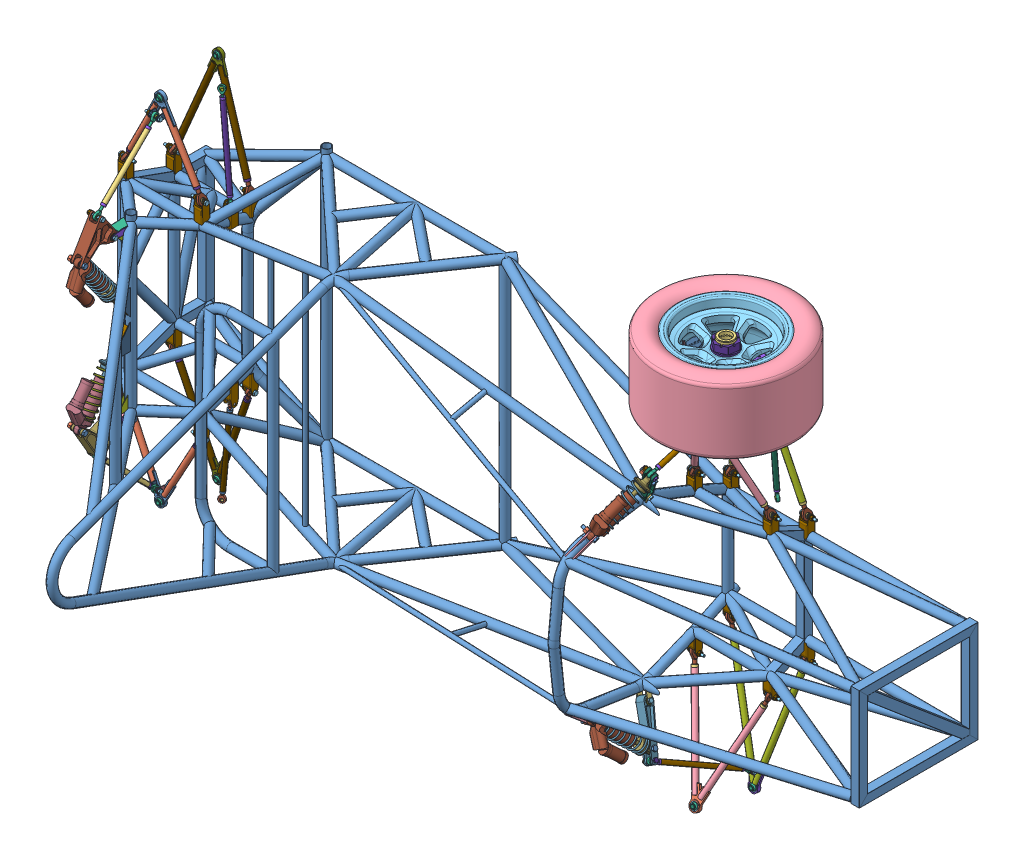
SolidWorks assembly AE-Rolling Chassis Assembly, configuration Default. Lengths in mm.
Overall size (2356.42 1252.94 1211.91).
496 component instances, 112 part files, 12 mates.
Components (placement in the parent):
- FR-A0100-FG_3-Space_Frame-1: FR-A0100-FG_3-Space_Frame [Default<As Machined>] at origin size (2341.42 791.46 1187.78)
- SP-A0200-AD-Front Axle Assembly-1: SP-A0200-AD-Front Axle Assembly [Default] at (231.003 -38.1001 -73.813) x (1 0 0) z (0 0 1) size (283.43 1142.4 502.75)
  - Upper A-Arm^SP-A0200-AD-Front Axle Assembly-1: Upper A-Arm^SP-A0200-AD-Front Axle Assembly [Default] at (0 340.1778 -103.3743) x (1 0 0) z (0 -0.807933 0.589274) size (223.78 263.64 179.68) (virtual)
    - SP-Upper Apex Front-1: SP-Upper Apex Front [Default] at (789.6198 444.1063 49.8797) x (0.938572 -0.289882 0.187221) z (0 0.542537 0.840032) size (51.11 64.07 9.53)
    - SP-10003-AD-Threaded Insert-1: SP-10003-AD-Threaded Insert [A-Arm] at (690.6588 218.0055 195.9078) x (-0.938572 0.289882 -0.187221) z (-0.345084 -0.78843 0.50921) size (15.88 15.88 15.88)
    - SP-10003-AD-Threaded Insert-2: SP-10003-AD-Threaded Insert [A-Arm] at (888.5808 218.0055 195.9078) x (0 0.542537 0.840032) z (0.345084 -0.78843 0.50921) size (15.88 15.88 15.88)
    - SP-Upper A-Arm Tube-1: SP-Upper A-Arm Tube [Default] at (732.4698 313.533 134.2109) x (0 -0.542537 -0.840032) z (0.938572 -0.289882 0.187221) size (15.88 272.31 15.88)
    - SP-Upper A-Arm Tube-2: SP-Upper A-Arm Tube [Default] at (846.7698 313.533 134.2109) x (0 0.542537 0.840032) z (-0.938572 -0.289882 0.187221) size (15.88 272.31 15.88)
    - FS-HIGH MISALIGN SPHERICAL BEARING, 0.375-0.906D (3072-6G)-1: FS-HIGH MISALIGN SPHERICAL BEARING, 0.375-0.906D (3072-6G) [Default] at (789.6198 444.1063 49.8797) x (-0.345084 -0.78843 0.50921) z (-0.938572 0.289882 -0.187221) size (26.46 21.71 26.13)
      - Race^FS-HIGH MISALIGN SPHERICAL BEARING, 0.375-0.906D (3072-6G)-1: Race^FS-HIGH MISALIGN SPHERICAL BEARING, 0.375-0.906D (3072-6G) [Default] at origin size (23.01 8.76 23.01) (virtual)
      - Ball^FS-HIGH MISALIGN SPHERICAL BEARING, 0.375-0.906D (3072-6G)-1: Ball^FS-HIGH MISALIGN SPHERICAL BEARING, 0.375-0.906D (3072-6G) [Default] x (0.359576 -0.008176 0.93308) z (-0.932238 -0.046516 0.358844) size (19.84 20.65 19.84) (virtual)
  - Lower A-Arm^SP-A0200-AD-Front Axle Assembly-1: Lower A-Arm^SP-A0200-AD-Front Axle Assembly [Default] at (0 -0.114 0.1797) x (1 0 0) z (0 0.000904 1) size (226.81 360.38 61.75) (virtual)
    - SP-Front Lower A-Arm Tube-2: SP-Front Lower A-Arm Tube [Default] at (844.893 441.1433 99.9128) x (0.296605 -0.948118 -0.114444) z (0 -0.119836 0.992794) size (339.15 15.88 15.88)
    - SP-Lower Apex Front-1: SP-Lower Apex Front [Default] at (798.1748 590.481 117.9388) x (0.955 -0.294468 -0.035544) z (0 -0.119836 0.992794) size (48.15 64.07 9.53)
    - SP-10003-AD-Threaded Insert-1: SP-10003-AD-Threaded Insert [A-Arm] at (899.2907 267.2577 78.9237) x (0.955 0.294468 0.035544) z (0.296605 -0.948118 -0.114444) size (15.88 15.88 15.88)
    - SP-10003-AD-Threaded Insert-2: SP-10003-AD-Threaded Insert [A-Arm] at (697.0589 267.2577 78.9237) x (0.955 -0.294468 -0.035544) z (-0.296605 -0.948118 -0.114444) size (15.88 15.88 15.88)
    - FS-HIGH MISALIGN SPHERICAL BEARING, 0.375-0.906D (3072-6G)-1: FS-HIGH MISALIGN SPHERICAL BEARING, 0.375-0.906D (3072-6G) [Default] at (798.1748 590.481 117.9388) x (0.296605 0.948118 0.114444) z (-0.955 0.294468 0.035544) size (26.46 21.71 26.13)
      - Race^FS-HIGH MISALIGN SPHERICAL BEARING, 0.375-0.906D (3072-6G)-1: Race^FS-HIGH MISALIGN SPHERICAL BEARING, 0.375-0.906D (3072-6G) [Default] at origin size (23.01 8.76 23.01) (virtual)
      - Ball^FS-HIGH MISALIGN SPHERICAL BEARING, 0.375-0.906D (3072-6G)-1: Ball^FS-HIGH MISALIGN SPHERICAL BEARING, 0.375-0.906D (3072-6G) [Default] x (0.359576 -0.008176 0.93308) z (-0.932238 -0.046516 0.358844) size (19.84 20.65 19.84) (virtual)
    - SP-Front Lower A-Arm Tube-3: SP-Front Lower A-Arm Tube [Default] at (751.4566 441.1433 99.9128) x (-0.296605 -0.948118 -0.114444) z (0 -0.119836 0.992794) size (339.15 15.88 15.88)
  - SP-C30066-AA-A-Arm Tab Box-2: SP-C30066-AA-A-Arm Tab Box [Default] at (903.9198 253.9613 173.2262) x (0 1 0) z (0 0 -1) size (60.32 25.4 25.4)
  - SP-C30066-AA-A-Arm Tab Box-3: SP-C30066-AA-A-Arm Tab Box [Default] at (675.3198 253.9613 173.2262) x (0 1 0) z (0 0 -1) size (60.32 25.4 25.4)
  - SP-C30066-AA-A-Arm Tab Box-4: SP-C30066-AA-A-Arm Tab Box [Default] at (912.4748 207.6041 73.8128) x (0 1 0) z (0 0 -1) size (60.32 25.4 25.4)
  - SP-C30066-AA-A-Arm Tab Box-5: SP-C30066-AA-A-Arm Tab Box [Default] at (683.8748 207.6066 73.5172) x (0 0.999857 0.016927) z (0 0.016927 -0.999857) size (60.32 25.4 25.4)
  - SP-30063-AB- Front Pushrod Tab-1: SP-30063-AB- Front Pushrod Tab [Default] at (810.0811 539.62 115.4288) x (1 0 0) z (0 0.104591 -0.994515) size (1.59 15.88 23.81)
  - SP-30063-AB- Front Pushrod Tab-2: SP-30063-AB- Front Pushrod Tab [Default] at (786.2686 539.62 115.4288) x (1 0 0) z (0 0.104591 -0.994515) size (1.59 15.88 23.81)
  - SP-A0105-AC-Ohlin TTX25 MKII, 200mm-2: SP-A0105-AC-Ohlin TTX25 MKII, 200mm [Default] at (696.4401 277.6233 502.0343) x (0.862886 -0.493364 -0.109636) z (-0.277169 -0.64335 0.713637) size (48.39 85.02 197.6)
    - Shock Body^SP-A0105-AC-Ohlin TTX25 MKII, 200mm-1: Shock Body^SP-A0105-AC-Ohlin TTX25 MKII, 200mm [Default] at origin size (40.76 80 131.7) (virtual)
    - Head^SP-A0105-AC-Ohlin TTX25 MKII, 200mm-1: Head^SP-A0105-AC-Ohlin TTX25 MKII, 200mm [Default] at (0 0 -174.6) size (46 46 119) (virtual)
    - Ball^SP-A0105-AC-Ohlin TTX25 MKII, 200mm-1: Ball^SP-A0105-AC-Ohlin TTX25 MKII, 200mm [Default] at (0 0 -174.6) x (-0.011681 0.107343 0.994153) z (0.993776 0.111394 -0.000351) size (15 15 8) (virtual)
    - Ball^SP-A0105-AC-Ohlin TTX25 MKII, 200mm-2: Ball^SP-A0105-AC-Ohlin TTX25 MKII, 200mm [Default] x (0.079523 -0.862756 -0.499328) z (0.965926 -0.057074 0.252448) size (15 15 8) (virtual)
    - SP-#####-AB-Spring-1: SP-#####-AB-Spring [Default] at (0 0 -151.1) size (48.39 49.05 127.97)
  - Front Rocker Assembly-1: Front Rocker Assembly [Default] at (694.2782 309.5507 341.3462) x (0.862886 -0.493364 -0.109636) z (-0.088476 -0.361041 0.928343) size (45.3 150.81 28.57)
    - SP-Front Rocker-1: SP-Front Rocker [Default] at origin size (25.4 150.81 28.57)
    - FS-BALL BEARING, 0.25ID-0.75OD (60355K702)-1: FS-BALL BEARING, 0.25ID-0.75OD (60355K702) [Default] at (9.1281 0 0) x (0 0 1) z (-1 0 0) size (19.05 19.05 7.14)
    - FS-BALL BEARING, 0.25ID-0.75OD (60355K702)-2: FS-BALL BEARING, 0.25ID-0.75OD (60355K702) [Default] at (-9.1281 0 0) x (0 0 1) z (-1 0 0) size (19.05 19.05 7.14)
    - FS-CADMIUM PLATED C3 HX, 0.25x28-1.41-0.469 (AN4-13A)-1: FS-CADMIUM PLATED C3 HX, 0.25x28-1.41-0.469 (AN4-13A) [Default] at (-3.0226 127 0) x (-1 0 0) z (0 1 0) size (40.18 12.9 11.18)
    - FS-NYLOC G8 HX, 0.25x28-0.3125 (90630A145)-1: FS-NYLOC G8 HX, 0.25x28-0.3125 (90630A145) [Default] at (-12.7 127 0) x (0 1 0) z (0 0 1) size (11.11 7.94 12.83)
    - FS-ZINC YELLOW CHROMATE C10.9 HX, M8x1.25-40-22 (95327A569)-1: FS-ZINC YELLOW CHROMATE C10.9 HX, M8x1.25-40-22 (95327A569) [Default] at (-4.65 101.6 0) x (-1 0 0) z (0 0 1) size (45.3 15.01 13)
    - FS-NYLOC FLHX C8, M8x1.25-11.1 (92461A400)-1: FS-NYLOC FLHX C8, M8x1.25-11.1 (92461A400) [Default] at (-23.8 101.6 0) x (0 1 0) z (-1 0 0) size (17.9 17.9 11.1)
  - SP-A0200-Front Rocker Tab Box-1: SP-A0200-Front Rocker Tab Box [Front] at (706.6066 302.5017 339.7797) x (0.862886 -0.493364 -0.109636) z (-0.497595 -0.791354 -0.355188) size (3.17 19.05 44.54)
  - SP-A0200-Front Rocker Tab Box-2: SP-A0200-Front Rocker Tab Box [Front] at (681.9497 316.5996 342.9126) x (0.862886 -0.493364 -0.109636) z (-0.497595 -0.791354 -0.355188) size (3.17 19.05 44.54)
  - SP-A0200-Shock Tab-1: SP-A0200-Shock Tab [Default] at (703.1358 273.795 501.1836) x (0.862886 -0.493364 -0.109636) z (-0.277169 -0.64335 0.713637) size (3.17 23.81 77.22)
  - SP-A0200-Shock Tab-2: SP-A0200-Shock Tab [Default] at (689.4375 281.6271 502.9241) x (0.862886 -0.493364 -0.109636) z (-0.277169 -0.64335 0.713637) size (3.17 23.81 77.22)
  - FS-NYLOC G8 HX, 0.25x28-0.3125 (90630A145)-3: FS-NYLOC G8 HX, 0.25x28-0.3125 (90630A145) [Default] at (688.0198 271.4238 173.2262) x (0 0 -1) z (0 -1 0) size (11.11 7.94 12.83)
  - FS-NYLOC G8 HX, 0.25x28-0.3125 (90630A145)-4: FS-NYLOC G8 HX, 0.25x28-0.3125 (90630A145) [Default] at (696.5748 225.0666 73.8128) x (0 0 1) z (0 1 0) size (11.11 7.94 12.83)
  - FS-CADMIUM PLATED C3 HEX, 0.25x28-1.65-0.469 (AN4-13A)-1: FS-CADMIUM PLATED C3 HEX, 0.25x28-1.65-0.469 (AN4-13A) [Default] at (909.9904 271.4238 173.2262) size (46.28 12.9 11.18)
  - FS-CADMIUM PLATED C3 HEX, 0.25x28-1.65-0.469 (AN4-13A)-2: FS-CADMIUM PLATED C3 HEX, 0.25x28-1.65-0.469 (AN4-13A) [Default] at (681.3904 271.4238 173.2262) size (46.28 12.9 11.18)
  - FS-CADMIUM PLATED C3 HEX, 0.25x28-1.65-0.469 (AN4-13A)-3: FS-CADMIUM PLATED C3 HEX, 0.25x28-1.65-0.469 (AN4-13A) [Default] at (689.9454 225.0666 73.8128) size (46.28 12.9 11.18)
  - FS-CADMIUM PLATED C3 HEX, 0.25x28-1.65-0.469 (AN4-13A)-4: FS-CADMIUM PLATED C3 HEX, 0.25x28-1.65-0.469 (AN4-13A) [Default] at (918.5454 225.0666 73.8128) size (46.28 12.9 11.18)
  - FS-CADMIUM PLATED C3 HEX, 0.25x28-1.65-0.469 (AN4-13A)-5: FS-CADMIUM PLATED C3 HEX, 0.25x28-1.65-0.469 (AN4-13A) [Default] at (792.898 537.9596 131.2167) x (-1 0 0) z (0 0.104591 -0.994515) size (46.28 12.9 11.18)
  - FS-CADMIUM PLATED C3 HEX, 0.25x28-1.65-0.469 (AN4-13A)-6: FS-CADMIUM PLATED C3 HEX, 0.25x28-1.65-0.469 (AN4-13A) [Default] at (691.7796 310.9792 341.6636) x (-0.862886 0.493364 0.109636) z (0.505399 0.842338 0.187186) size (46.28 12.9 11.18)
  - FS-ZINC YELLOW CHROMATE C10.9 HX, M8x1.25-40-22 (95327A569)-1: FS-ZINC YELLOW CHROMATE C10.9 HX, M8x1.25-40-22 (95327A569) [Default] at (689.5346 281.5716 502.9117) x (-0.862886 0.493364 0.109636) z (0.422618 0.5854 0.691883) size (45.3 15.01 13)
  - FS-NYLOC FLHX C8, M8x1.25-11.1 (92461A400)-1: FS-NYLOC FLHX C8, M8x1.25-11.1 (92461A400) [Default] at (678.4896 287.8867 504.3151) x (-0.277169 -0.64335 0.713637) z (-0.862886 0.493364 0.109636) size (17.9 17.9 11.1)
  - FS-NYLOC G8 HX, 0.25x28-0.3125 (90630A145)-1: FS-NYLOC G8 HX, 0.25x28-0.3125 (90630A145) [Default] at (916.6198 271.4238 173.2262) x (0 0 -1) z (0 -1 0) size (11.11 7.94 12.83)
  - FS-NYLOC G8 HX, 0.25x28-0.3125 (90630A145)-2: FS-NYLOC G8 HX, 0.25x28-0.3125 (90630A145) [Default] at (925.1748 225.0666 73.8128) x (0 0 1) z (0 1 0) size (11.11 7.94 12.83)
  - FS-NYLOC G8 HX, 0.25x28-0.3125 (90630A145)-5: FS-NYLOC G8 HX, 0.25x28-0.3125 (90630A145) [Default] at (786.2686 537.9596 131.2167) x (0 0.994515 0.104591) z (0 -0.104591 0.994515) size (11.11 7.94 12.83)
  - Push Rod^SP-A0200-AD-Front Axle Assembly-1: Push Rod^SP-A0200-AD-Front Axle Assembly [Default] at (-77.4197 117.9369 116.0221) x (0.981785 -0.1411 -0.127232) z (0.129346 0.005872 0.991582) size (77.15 168.18 273.97) (virtual)
    - FS-MALE ROD END UNF-3A, 0.25x28-0.25D (AM-4)-1: FS-MALE ROD END UNF-3A, 0.25x28-0.25D (AM-4) [Default] at (744.0599 398.8817 377.8613) x (-0.313321 -0.797417 -0.515709) z (0.188596 0.479987 -0.856764) size (19.32 14.06 49.44)
      - Body^FS-MALE ROD END UNF-3A, 0.25x28-0.25D (AM-4)-2: Body^FS-MALE ROD END UNF-3A, 0.25x28-0.25D (AM-4) [Default] at origin size (19.32 7.2 49.44) (virtual)
      - Ball^FS-MALE ROD END UNF-3A, 0.25x28-0.25D (AM-4)-2: Ball^FS-MALE ROD END UNF-3A, 0.25x28-0.25D (AM-4) [Default] x (0.09633 0.218783 0.971007) z (-0.984027 0.167661 0.059845) size (12.7 9.53 12.7) (virtual)
    - FS-MALE ROD END UNF-3A, 0.25x28-0.25D (AM-4)-2: FS-MALE ROD END UNF-3A, 0.25x28-0.25D (AM-4) [Default] at (798.4475 537.3007 130.7871) x (0.310336 0.78982 0.529034) z (-0.193469 -0.492388 0.848601) size (19.32 14.06 49.44)
      - Body^FS-MALE ROD END UNF-3A, 0.25x28-0.25D (AM-4)-2: Body^FS-MALE ROD END UNF-3A, 0.25x28-0.25D (AM-4) [Default] at origin size (19.32 7.2 49.44) (virtual)
      - Ball^FS-MALE ROD END UNF-3A, 0.25x28-0.25D (AM-4)-2: Ball^FS-MALE ROD END UNF-3A, 0.25x28-0.25D (AM-4) [Default] x (0.09633 0.218783 0.971007) z (-0.984027 0.167661 0.059845) size (12.7 9.53 12.7) (virtual)
    - SP-10003-AC-Threaded Insert-1: SP-10003-AC-Threaded Insert [AM-4 Rod End Thread] at (750.6466 415.6452 347.9388) x (0.313321 0.797417 0.515709) z (-0.188596 -0.479987 0.856764) size (12.7 12.7 15.88)
    - SP-10003-AC-Threaded Insert-2: SP-10003-AC-Threaded Insert [AM-4 Rod End Thread] at (791.691 520.1052 160.4226) x (-0.310336 -0.78982 -0.529034) z (0.193469 0.492388 -0.848601) size (12.7 12.7 15.88)
    - SP-A0200-Front Push Rod Tube-1: SP-A0200-Front Push Rod Tube [Default] at (771.2537 468.0912 254.3242) x (-0.313321 -0.797417 -0.515709) z (0.930732 -0.365703 0) size (12.7 237.68 12.7)
  - FS-ROD END RETAINING WASHER, 0.25-0.245 (NO PN)-1: FS-ROD END RETAINING WASHER, 0.25-0.245 (NO PN) [Default] at (923.7143 225.0666 73.8128) x (0 0 1) z (-1 0 0) size (12.7 12.7 6.22)
  - FS-ROD END RETAINING WASHER, 0.25-0.245 (NO PN)-2: FS-ROD END RETAINING WASHER, 0.25-0.245 (NO PN) [Default] at (901.2353 225.0666 73.8128) x (0 0 -1) z (1 0 0) size (12.7 12.7 6.22)
  - FS-ROD END RETAINING WASHER, 0.25-0.245 (NO PN)-3: FS-ROD END RETAINING WASHER, 0.25-0.245 (NO PN) [Default] at (915.1593 271.4238 173.2262) x (0 0 -1) z (-1 0 0) size (12.7 12.7 6.22)
  - FS-ROD END RETAINING WASHER, 0.25-0.245 (NO PN)-4: FS-ROD END RETAINING WASHER, 0.25-0.245 (NO PN) [Default] at (892.6803 271.4238 173.2262) x (0 0 1) z (1 0 0) size (12.7 12.7 6.22)
  - FS-ROD END RETAINING WASHER, 0.25-0.245 (NO PN)-5: FS-ROD END RETAINING WASHER, 0.25-0.245 (NO PN) [Default] at (695.1143 225.0666 73.8128) x (0 0 1) z (-1 0 0) size (12.7 12.7 6.22)
  - FS-ROD END RETAINING WASHER, 0.25-0.245 (NO PN)-6: FS-ROD END RETAINING WASHER, 0.25-0.245 (NO PN) [Default] at (672.6353 225.0666 73.8128) x (0 0 -1) z (1 0 0) size (12.7 12.7 6.22)
  - FS-ROD END RETAINING WASHER, 0.25-0.245 (NO PN)-7: FS-ROD END RETAINING WASHER, 0.25-0.245 (NO PN) [Default] at (686.5593 271.4238 173.2262) x (0 0 -1) z (-1 0 0) size (12.7 12.7 6.22)
  - FS-ROD END RETAINING WASHER, 0.25-0.245 (NO PN)-8: FS-ROD END RETAINING WASHER, 0.25-0.245 (NO PN) [Default] at (664.0803 271.4238 173.2262) x (0 0 1) z (1 0 0) size (12.7 12.7 6.22)
  - FS-ROD END RETAINING WASHER, 0.25-0.245 (NO PN)-9: FS-ROD END RETAINING WASHER, 0.25-0.245 (NO PN) [Default] at (810.2081 537.9596 131.2167) x (0 0.994515 0.104591) z (-1 0 0) size (12.7 12.7 6.22)
  - FS-ROD END RETAINING WASHER, 0.25-0.245 (NO PN)-10: FS-ROD END RETAINING WASHER, 0.25-0.245 (NO PN) [Default] at (787.7291 537.9596 131.2167) x (0 -0.994515 -0.104591) z (1 0 0) size (12.7 12.7 6.22)
  - FS-MALE ROD END UNJF-3A, 0.375x24-0.25D (HXAM-4T)-1: FS-MALE ROD END UNJF-3A, 0.375x24-0.25D (HXAM-4T) [Simplified] at (675.3198 271.4238 173.2262) x (0.013325 0.354377 -0.935008) z (0.345084 0.876009 0.336934) size (26.22 15.06 62.54)
    - Body^FS-MALE ROD END UNJF-3A, 0.375x24-0.25D (HXAM-4T)-1: Body^FS-MALE ROD END UNJF-3A, 0.375x24-0.25D (HXAM-4T) [no_threads] at origin size (26.22 9.62 62.54)
    - Ball^FS-MALE ROD END UNJF-3A, 0.375x24-0.25D (HXAM-4T)-1: Ball^FS-MALE ROD END UNJF-3A, 0.375x24-0.25D (HXAM-4T) [Default] at origin size (15.06 15.06 15.06)
  - FS-MALE ROD END UNJF-3A, 0.375x24-0.25D (HXAM-4T)-2: FS-MALE ROD END UNJF-3A, 0.375x24-0.25D (HXAM-4T) [Simplified] at (903.9198 271.4238 173.2262) x (0.045305 -0.343021 0.938235) z (-0.345084 0.876009 0.336934) size (26.22 15.06 62.54)
    - Body^FS-MALE ROD END UNJF-3A, 0.375x24-0.25D (HXAM-4T)-1: Body^FS-MALE ROD END UNJF-3A, 0.375x24-0.25D (HXAM-4T) [no_threads] at origin size (26.22 9.62 62.54)
    - Ball^FS-MALE ROD END UNJF-3A, 0.375x24-0.25D (HXAM-4T)-1: Ball^FS-MALE ROD END UNJF-3A, 0.375x24-0.25D (HXAM-4T) [Default] at origin size (15.06 15.06 15.06)
  - FS-MALE ROD END UNJF-3A, 0.375x24-0.25D (HXAM-4T)-3: FS-MALE ROD END UNJF-3A, 0.375x24-0.25D (HXAM-4T) [Simplified] at (683.8748 225.0666 73.8128) x (0.051295 0.102949 -0.993363) z (0.296605 0.948221 0.113586) size (26.22 15.06 62.54)
    - Body^FS-MALE ROD END UNJF-3A, 0.375x24-0.25D (HXAM-4T)-1: Body^FS-MALE ROD END UNJF-3A, 0.375x24-0.25D (HXAM-4T) [no_threads] at origin size (26.22 9.62 62.54)
    - Ball^FS-MALE ROD END UNJF-3A, 0.375x24-0.25D (HXAM-4T)-1: Ball^FS-MALE ROD END UNJF-3A, 0.375x24-0.25D (HXAM-4T) [Default] at origin size (15.06 15.06 15.06)
  - FS-MALE ROD END UNJF-3A, 0.375x24-0.25D (HXAM-4T)-4: FS-MALE ROD END UNJF-3A, 0.375x24-0.25D (HXAM-4T) [Simplified] at (912.4748 225.0666 73.8128) x (0.102858 0.149966 -0.983326) z (-0.296605 0.948221 0.113586) size (26.22 15.06 62.54)
    - Body^FS-MALE ROD END UNJF-3A, 0.375x24-0.25D (HXAM-4T)-1: Body^FS-MALE ROD END UNJF-3A, 0.375x24-0.25D (HXAM-4T) [no_threads] at origin size (26.22 9.62 62.54)
    - Ball^FS-MALE ROD END UNJF-3A, 0.375x24-0.25D (HXAM-4T)-1: Ball^FS-MALE ROD END UNJF-3A, 0.375x24-0.25D (HXAM-4T) [Default] at origin size (15.06 15.06 15.06)
  - FS-NYLOC G8 HX, 0.25x28-0.3125 (90630A145)-6: FS-NYLOC G8 HX, 0.25x28-0.3125 (90630A145) [Default] at (925.1748 -148.8666 73.8128) x (0 0 1) z (0 1 0) size (11.11 7.94 12.83)
  - FS-CADMIUM PLATED C3 HEX, 0.25x28-1.65-0.469 (AN4-13A)-7: FS-CADMIUM PLATED C3 HEX, 0.25x28-1.65-0.469 (AN4-13A) [Default] at (792.898 -461.7596 131.2167) x (-1 0 0) z (0 0.104591 0.994515) size (46.28 12.9 11.18)
  - FS-CADMIUM PLATED C3 HEX, 0.25x28-1.65-0.469 (AN4-13A)-8: FS-CADMIUM PLATED C3 HEX, 0.25x28-1.65-0.469 (AN4-13A) [Default] at (691.7796 -234.7792 341.6636) x (-0.862886 -0.493364 0.109636) z (-0.505399 0.842338 -0.187186) size (46.28 12.9 11.18)
  - FS-ROD END RETAINING WASHER, 0.25-0.245 (NO PN)-11: FS-ROD END RETAINING WASHER, 0.25-0.245 (NO PN) [Default] at (672.6353 -148.8666 73.8128) x (0 0 1) z (1 0 0) size (12.7 12.7 6.22)
  - FS-ROD END RETAINING WASHER, 0.25-0.245 (NO PN)-12: FS-ROD END RETAINING WASHER, 0.25-0.245 (NO PN) [Default] at (901.2353 -148.8666 73.8128) x (0 0 1) z (1 0 0) size (12.7 12.7 6.22)
  - FS-NYLOC G8 HX, 0.25x28-0.3125 (90630A145)-7: FS-NYLOC G8 HX, 0.25x28-0.3125 (90630A145) [Default] at (696.5748 -148.8666 73.8128) x (0 0 1) z (0 1 0) size (11.11 7.94 12.83)
  - FS-NYLOC FLHX C8, M8x1.25-11.1 (92461A400)-2: FS-NYLOC FLHX C8, M8x1.25-11.1 (92461A400) [Default] at (678.4896 -211.6867 504.3151) x (0.277169 -0.64335 -0.713637) z (-0.862886 -0.493364 0.109636) size (17.9 17.9 11.1)
  - FS-NYLOC G8 HX, 0.25x28-0.3125 (90630A145)-8: FS-NYLOC G8 HX, 0.25x28-0.3125 (90630A145) [Default] at (688.0198 -195.2238 173.2262) x (0 0 -1) z (0 -1 0) size (11.11 7.94 12.83)
  - FS-CADMIUM PLATED C3 HEX, 0.25x28-1.65-0.469 (AN4-13A)-9: FS-CADMIUM PLATED C3 HEX, 0.25x28-1.65-0.469 (AN4-13A) [Default] at (918.5454 -148.8666 73.8128) x (1 0 0) z (0 0 -1) size (46.28 12.9 11.18)
  - FS-CADMIUM PLATED C3 HEX, 0.25x28-1.65-0.469 (AN4-13A)-10: FS-CADMIUM PLATED C3 HEX, 0.25x28-1.65-0.469 (AN4-13A) [Default] at (909.9904 -195.2238 173.2262) x (1 0 0) z (0 0 -1) size (46.28 12.9 11.18)
  - FS-ROD END RETAINING WASHER, 0.25-0.245 (NO PN)-13: FS-ROD END RETAINING WASHER, 0.25-0.245 (NO PN) [Default] at (695.1143 -148.8666 73.8128) x (0 0 -1) z (-1 0 0) size (12.7 12.7 6.22)
  - FS-NYLOC G8 HX, 0.25x28-0.3125 (90630A145)-9: FS-NYLOC G8 HX, 0.25x28-0.3125 (90630A145) [Default] at (916.6198 -195.2238 173.2262) x (0 0 -1) z (0 -1 0) size (11.11 7.94 12.83)
  - FS-ROD END RETAINING WASHER, 0.25-0.245 (NO PN)-14: FS-ROD END RETAINING WASHER, 0.25-0.245 (NO PN) [Default] at (923.7143 -148.8666 73.8128) x (0 0 -1) z (-1 0 0) size (12.7 12.7 6.22)
  - FS-ROD END RETAINING WASHER, 0.25-0.245 (NO PN)-15: FS-ROD END RETAINING WASHER, 0.25-0.245 (NO PN) [Default] at (892.6803 -195.2238 173.2262) x (0 0 -1) z (1 0 0) size (12.7 12.7 6.22)
  - FS-ROD END RETAINING WASHER, 0.25-0.245 (NO PN)-16: FS-ROD END RETAINING WASHER, 0.25-0.245 (NO PN) [Default] at (915.1593 -195.2238 173.2262) x (0 0 1) z (-1 0 0) size (12.7 12.7 6.22)
  - Push Rod^SP-A0200-AD-Front Axle Assembly-2: Push Rod^SP-A0200-AD-Front Axle Assembly [Default] at (1633.0862 -753.9206 401.5957) x (-0.981785 -0.1411 0.127232) z (-0.129346 0.005872 -0.991582) size (77.15 168.18 273.97) (virtual)
    - FS-MALE ROD END UNF-3A, 0.25x28-0.25D (AM-4)-1: FS-MALE ROD END UNF-3A, 0.25x28-0.25D (AM-4) [Default] at (744.0599 398.8817 377.8613) x (-0.313321 -0.797417 -0.515709) z (0.188596 0.479987 -0.856764) size (19.32 14.06 49.44)
      - Body^FS-MALE ROD END UNF-3A, 0.25x28-0.25D (AM-4)-2: Body^FS-MALE ROD END UNF-3A, 0.25x28-0.25D (AM-4) [Default] at origin size (19.32 7.2 49.44) (virtual)
      - Ball^FS-MALE ROD END UNF-3A, 0.25x28-0.25D (AM-4)-2: Ball^FS-MALE ROD END UNF-3A, 0.25x28-0.25D (AM-4) [Default] x (0.09633 0.218783 0.971007) z (-0.984027 0.167661 0.059845) size (12.7 9.53 12.7) (virtual)
    - FS-MALE ROD END UNF-3A, 0.25x28-0.25D (AM-4)-2: FS-MALE ROD END UNF-3A, 0.25x28-0.25D (AM-4) [Default] at (798.4475 537.3007 130.7871) x (0.310336 0.78982 0.529034) z (-0.193469 -0.492388 0.848601) size (19.32 14.06 49.44)
      - Body^FS-MALE ROD END UNF-3A, 0.25x28-0.25D (AM-4)-2: Body^FS-MALE ROD END UNF-3A, 0.25x28-0.25D (AM-4) [Default] at origin size (19.32 7.2 49.44) (virtual)
      - Ball^FS-MALE ROD END UNF-3A, 0.25x28-0.25D (AM-4)-2: Ball^FS-MALE ROD END UNF-3A, 0.25x28-0.25D (AM-4) [Default] x (0.09633 0.218783 0.971007) z (-0.984027 0.167661 0.059845) size (12.7 9.53 12.7) (virtual)
    - SP-10003-AC-Threaded Insert-1: SP-10003-AC-Threaded Insert [AM-4 Rod End Thread] at (750.6466 415.6452 347.9388) x (0.313321 0.797417 0.515709) z (-0.188596 -0.479987 0.856764) size (12.7 12.7 15.88)
    - SP-10003-AC-Threaded Insert-2: SP-10003-AC-Threaded Insert [AM-4 Rod End Thread] at (791.691 520.1052 160.4226) x (-0.310336 -0.78982 -0.529034) z (0.193469 0.492388 -0.848601) size (12.7 12.7 15.88)
    - SP-A0200-Front Push Rod Tube-1: SP-A0200-Front Push Rod Tube [Default] at (771.2537 468.0912 254.3242) x (-0.313321 -0.797417 -0.515709) z (0.930732 -0.365703 0) size (12.7 237.68 12.7)
  - FS-ZINC YELLOW CHROMATE C10.9 HX, M8x1.25-40-22 (95327A569)-2: FS-ZINC YELLOW CHROMATE C10.9 HX, M8x1.25-40-22 (95327A569) [Default] at (689.5346 -205.3716 502.9117) x (-0.862886 -0.493364 0.109636) z (-0.422618 0.5854 -0.691883) size (45.3 15.01 13)
  - FS-CADMIUM PLATED C3 HEX, 0.25x28-1.65-0.469 (AN4-13A)-11: FS-CADMIUM PLATED C3 HEX, 0.25x28-1.65-0.469 (AN4-13A) [Default] at (681.3904 -195.2238 173.2262) x (1 0 0) z (0 0 -1) size (46.28 12.9 11.18)
  - FS-CADMIUM PLATED C3 HEX, 0.25x28-1.65-0.469 (AN4-13A)-12: FS-CADMIUM PLATED C3 HEX, 0.25x28-1.65-0.469 (AN4-13A) [Default] at (689.9454 -148.8666 73.8128) x (1 0 0) z (0 0 -1) size (46.28 12.9 11.18)
  - FS-ROD END RETAINING WASHER, 0.25-0.245 (NO PN)-17: FS-ROD END RETAINING WASHER, 0.25-0.245 (NO PN) [Default] at (787.7291 -461.7596 131.2167) x (0 -0.994515 0.104591) z (1 0 0) size (12.7 12.7 6.22)
  - FS-ROD END RETAINING WASHER, 0.25-0.245 (NO PN)-18: FS-ROD END RETAINING WASHER, 0.25-0.245 (NO PN) [Default] at (810.2081 -461.7596 131.2167) x (0 0.994515 -0.104591) z (-1 0 0) size (12.7 12.7 6.22)
  - FS-ROD END RETAINING WASHER, 0.25-0.245 (NO PN)-19: FS-ROD END RETAINING WASHER, 0.25-0.245 (NO PN) [Default] at (664.0803 -195.2238 173.2262) x (0 0 -1) z (1 0 0) size (12.7 12.7 6.22)
  - FS-ROD END RETAINING WASHER, 0.25-0.245 (NO PN)-20: FS-ROD END RETAINING WASHER, 0.25-0.245 (NO PN) [Default] at (686.5593 -195.2238 173.2262) x (0 0 1) z (-1 0 0) size (12.7 12.7 6.22)
  - FS-NYLOC G8 HX, 0.25x28-0.3125 (90630A145)-10: FS-NYLOC G8 HX, 0.25x28-0.3125 (90630A145) [Default] at (786.2686 -461.7596 131.2167) x (0 -0.994515 0.104591) z (0 -0.104591 -0.994515) size (11.11 7.94 12.83)
  - FS-MALE ROD END UNJF-3A, 0.375x24-0.25D (HXAM-4T)-5: FS-MALE ROD END UNJF-3A, 0.375x24-0.25D (HXAM-4T) [Simplified] at (675.3198 -195.2238 173.2262) x (0.013325 -0.354377 -0.935008) z (0.345084 -0.876009 0.336934) size (26.22 15.06 62.54)
    - Body^FS-MALE ROD END UNJF-3A, 0.375x24-0.25D (HXAM-4T)-1: Body^FS-MALE ROD END UNJF-3A, 0.375x24-0.25D (HXAM-4T) [no_threads] at origin size (26.22 9.62 62.54)
    - Ball^FS-MALE ROD END UNJF-3A, 0.375x24-0.25D (HXAM-4T)-1: Ball^FS-MALE ROD END UNJF-3A, 0.375x24-0.25D (HXAM-4T) [Default] at origin size (15.06 15.06 15.06)
  - FS-MALE ROD END UNJF-3A, 0.375x24-0.25D (HXAM-4T)-6: FS-MALE ROD END UNJF-3A, 0.375x24-0.25D (HXAM-4T) [Simplified] at (683.8748 -148.8666 73.8128) x (0.051295 -0.102949 -0.993363) z (0.296605 -0.948221 0.113586) size (26.22 15.06 62.54)
    - Body^FS-MALE ROD END UNJF-3A, 0.375x24-0.25D (HXAM-4T)-1: Body^FS-MALE ROD END UNJF-3A, 0.375x24-0.25D (HXAM-4T) [no_threads] at origin size (26.22 9.62 62.54)
    - Ball^FS-MALE ROD END UNJF-3A, 0.375x24-0.25D (HXAM-4T)-1: Ball^FS-MALE ROD END UNJF-3A, 0.375x24-0.25D (HXAM-4T) [Default] at origin size (15.06 15.06 15.06)
  - FS-MALE ROD END UNJF-3A, 0.375x24-0.25D (HXAM-4T)-7: FS-MALE ROD END UNJF-3A, 0.375x24-0.25D (HXAM-4T) [Simplified] at (912.4748 -148.8666 73.8128) x (0.102858 -0.149966 -0.983326) z (-0.296605 -0.948221 0.113586) size (26.22 15.06 62.54)
    - Body^FS-MALE ROD END UNJF-3A, 0.375x24-0.25D (HXAM-4T)-1: Body^FS-MALE ROD END UNJF-3A, 0.375x24-0.25D (HXAM-4T) [no_threads] at origin size (26.22 9.62 62.54)
    - Ball^FS-MALE ROD END UNJF-3A, 0.375x24-0.25D (HXAM-4T)-1: Ball^FS-MALE ROD END UNJF-3A, 0.375x24-0.25D (HXAM-4T) [Default] at origin size (15.06 15.06 15.06)
  - FS-MALE ROD END UNJF-3A, 0.375x24-0.25D (HXAM-4T)-8: FS-MALE ROD END UNJF-3A, 0.375x24-0.25D (HXAM-4T) [Simplified] at (903.9198 -195.2238 173.2262) x (0.045305 0.343021 0.938235) z (-0.345084 -0.876009 0.336934) size (26.22 15.06 62.54)
    - Body^FS-MALE ROD END UNJF-3A, 0.375x24-0.25D (HXAM-4T)-1: Body^FS-MALE ROD END UNJF-3A, 0.375x24-0.25D (HXAM-4T) [no_threads] at origin size (26.22 9.62 62.54)
    - Ball^FS-MALE ROD END UNJF-3A, 0.375x24-0.25D (HXAM-4T)-1: Ball^FS-MALE ROD END UNJF-3A, 0.375x24-0.25D (HXAM-4T) [Default] at origin size (15.06 15.06 15.06)
  - MirrorSP-30063-AB- Front Pushrod Tab-3: MirrorSP-30063-AB- Front Pushrod Tab [Default] at (786.2686 -463.42 115.4288) x (1 0 0) z (0 0.104591 0.994515) size (1.59 15.88 23.81)
  - MirrorSP-30063-AB- Front Pushrod Tab-4: MirrorSP-30063-AB- Front Pushrod Tab [Default] at (810.0811 -463.42 115.4288) x (1 0 0) z (0 0.104591 0.994515) size (1.59 15.88 23.81)
  - SP-C30066-AA-A-Arm Tab Box-6: SP-C30066-AA-A-Arm Tab Box [Default] at (675.3198 -177.7613 173.2262) x (0 -1 0) z (0 0 1) size (60.32 25.4 25.4)
  - SP-C30066-AA-A-Arm Tab Box-7: SP-C30066-AA-A-Arm Tab Box [Default] at (903.9198 -177.7613 173.2262) x (0 -1 0) z (0 0 1) size (60.32 25.4 25.4)
  - Lower A-Arm^SP-A0200-AD-Front Axle Assembly-2: Lower A-Arm^SP-A0200-AD-Front Axle Assembly [Default] at (1596.3496 76.314 0.1797) x (-1 0 0) z (0 -0.000904 1) size (226.81 360.38 61.75) (virtual)
    - SP-Front Lower A-Arm Tube-2: SP-Front Lower A-Arm Tube [Default] at (844.893 441.1433 99.9128) x (0.296605 -0.948118 -0.114444) z (0 -0.119836 0.992794) size (339.15 15.88 15.88)
    - SP-Lower Apex Front-1: SP-Lower Apex Front [Default] at (798.1748 590.481 117.9388) x (0.955 -0.294468 -0.035544) z (0 -0.119836 0.992794) size (48.15 64.07 9.53)
    - SP-10003-AD-Threaded Insert-1: SP-10003-AD-Threaded Insert [A-Arm] at (899.2907 267.2577 78.9237) x (0.955 0.294468 0.035544) z (0.296605 -0.948118 -0.114444) size (15.88 15.88 15.88)
    - SP-10003-AD-Threaded Insert-2: SP-10003-AD-Threaded Insert [A-Arm] at (697.0589 267.2577 78.9237) x (0.955 -0.294468 -0.035544) z (-0.296605 -0.948118 -0.114444) size (15.88 15.88 15.88)
    - FS-HIGH MISALIGN SPHERICAL BEARING, 0.375-0.906D (3072-6G)-1: FS-HIGH MISALIGN SPHERICAL BEARING, 0.375-0.906D (3072-6G) [Default] at (798.1748 590.481 117.9388) x (0.296605 0.948118 0.114444) z (-0.955 0.294468 0.035544) size (26.46 21.71 26.13)
      - Race^FS-HIGH MISALIGN SPHERICAL BEARING, 0.375-0.906D (3072-6G)-1: Race^FS-HIGH MISALIGN SPHERICAL BEARING, 0.375-0.906D (3072-6G) [Default] at origin size (23.01 8.76 23.01) (virtual)
      - Ball^FS-HIGH MISALIGN SPHERICAL BEARING, 0.375-0.906D (3072-6G)-1: Ball^FS-HIGH MISALIGN SPHERICAL BEARING, 0.375-0.906D (3072-6G) [Default] x (0.359576 -0.008176 0.93308) z (-0.932238 -0.046516 0.358844) size (19.84 20.65 19.84) (virtual)
    - SP-Front Lower A-Arm Tube-3: SP-Front Lower A-Arm Tube [Default] at (751.4566 441.1433 99.9128) x (-0.296605 -0.948118 -0.114444) z (0 -0.119836 0.992794) size (339.15 15.88 15.88)
  - Upper A-Arm^SP-A0200-AD-Front Axle Assembly-2: Upper A-Arm^SP-A0200-AD-Front Axle Assembly [Default] at (1579.2396 -263.9778 -103.3743) x (-1 0 0) z (0 0.807933 0.589274) size (223.78 263.64 179.68) (virtual)
    - SP-Upper Apex Front-1: SP-Upper Apex Front [Default] at (789.6198 444.1063 49.8797) x (0.938572 -0.289882 0.187221) z (0 0.542537 0.840032) size (51.11 64.07 9.53)
    - SP-10003-AD-Threaded Insert-1: SP-10003-AD-Threaded Insert [A-Arm] at (690.6588 218.0055 195.9078) x (-0.938572 0.289882 -0.187221) z (-0.345084 -0.78843 0.50921) size (15.88 15.88 15.88)
    - SP-10003-AD-Threaded Insert-2: SP-10003-AD-Threaded Insert [A-Arm] at (888.5808 218.0055 195.9078) x (0 0.542537 0.840032) z (0.345084 -0.78843 0.50921) size (15.88 15.88 15.88)
    - SP-Upper A-Arm Tube-1: SP-Upper A-Arm Tube [Default] at (732.4698 313.533 134.2109) x (0 -0.542537 -0.840032) z (0.938572 -0.289882 0.187221) size (15.88 272.31 15.88)
    - SP-Upper A-Arm Tube-2: SP-Upper A-Arm Tube [Default] at (846.7698 313.533 134.2109) x (0 0.542537 0.840032) z (-0.938572 -0.289882 0.187221) size (15.88 272.31 15.88)
    - FS-HIGH MISALIGN SPHERICAL BEARING, 0.375-0.906D (3072-6G)-1: FS-HIGH MISALIGN SPHERICAL BEARING, 0.375-0.906D (3072-6G) [Default] at (789.6198 444.1063 49.8797) x (-0.345084 -0.78843 0.50921) z (-0.938572 0.289882 -0.187221) size (26.46 21.71 26.13)
      - Race^FS-HIGH MISALIGN SPHERICAL BEARING, 0.375-0.906D (3072-6G)-1: Race^FS-HIGH MISALIGN SPHERICAL BEARING, 0.375-0.906D (3072-6G) [Default] at origin size (23.01 8.76 23.01) (virtual)
      - Ball^FS-HIGH MISALIGN SPHERICAL BEARING, 0.375-0.906D (3072-6G)-1: Ball^FS-HIGH MISALIGN SPHERICAL BEARING, 0.375-0.906D (3072-6G) [Default] x (0.359576 -0.008176 0.93308) z (-0.932238 -0.046516 0.358844) size (19.84 20.65 19.84) (virtual)
  - SP-A0200-Shock Tab-3: SP-A0200-Shock Tab [Default] at (703.1358 -197.595 501.1836) x (0.862886 0.493364 -0.109636) z (-0.277169 0.64335 0.713637) size (3.17 23.81 77.22)
  - MirrorFront Rocker Assembly-2: MirrorFront Rocker Assembly [Default] at (694.2782 -233.3507 341.3462) x (0.862886 0.493364 -0.109636) z (0.088476 -0.361041 -0.928343) size (45.3 150.81 28.57)
    - MirrorSP-Front Rocker-1: MirrorSP-Front Rocker [Default] at origin size (25.4 150.81 28.57)
    - FS-BALL BEARING, 0.25ID-0.75OD (60355K702)-1: FS-BALL BEARING, 0.25ID-0.75OD (60355K702) [Default] at (9.1281 0 0) x (0 0 1) z (-1 0 0) size (19.05 19.05 7.14)
    - FS-BALL BEARING, 0.25ID-0.75OD (60355K702)-2: FS-BALL BEARING, 0.25ID-0.75OD (60355K702) [Default] at (-9.1281 0 0) x (0 0 1) z (-1 0 0) size (19.05 19.05 7.14)
    - FS-CADMIUM PLATED C3 HX, 0.25x28-1.41-0.469 (AN4-13A)-1: FS-CADMIUM PLATED C3 HX, 0.25x28-1.41-0.469 (AN4-13A) [Default] at (-3.0226 127 0) x (-1 0 0) z (0 -1 0) size (40.18 12.9 11.18)
    - FS-NYLOC G8 HX, 0.25x28-0.3125 (90630A145)-1: FS-NYLOC G8 HX, 0.25x28-0.3125 (90630A145) [Default] at (-12.7 127 0) x (0 1 0) z (0 0 1) size (11.11 7.94 12.83)
    - FS-ZINC YELLOW CHROMATE C10.9 HX, M8x1.25-40-22 (95327A569)-1: FS-ZINC YELLOW CHROMATE C10.9 HX, M8x1.25-40-22 (95327A569) [Default] at (-4.65 101.6 0) x (-1 0 0) z (0 0 1) size (45.3 15.01 13)
    - FS-NYLOC FLHX C8, M8x1.25-11.1 (92461A400)-1: FS-NYLOC FLHX C8, M8x1.25-11.1 (92461A400) [Default] at (-23.8 101.6 0) x (0 -1 0) z (-1 0 0) size (17.9 17.9 11.1)
  - SP-C30066-AA-A-Arm Tab Box-8: SP-C30066-AA-A-Arm Tab Box [Default] at (683.8748 -131.4066 73.5172) x (0 -0.999857 0.016927) z (0 0.016927 0.999857) size (60.32 25.4 25.4)
  - SP-A0200-Shock Tab-4: SP-A0200-Shock Tab [Default] at (689.4375 -205.4271 502.9241) x (0.862886 0.493364 -0.109636) z (-0.277169 0.64335 0.713637) size (3.17 23.81 77.22)
  - SP-A0200-Front Rocker Tab Box-3: SP-A0200-Front Rocker Tab Box [Front] at (681.9497 -240.3996 342.9126) x (-0.862886 -0.493364 0.109636) z (-0.497595 0.791354 -0.355188) size (3.17 19.05 44.54)
  - SP-A0200-Front Rocker Tab Box-4: SP-A0200-Front Rocker Tab Box [Front] at (706.6066 -226.3017 339.7797) x (-0.862886 -0.493364 0.109636) z (-0.497595 0.791354 -0.355188) size (3.17 19.05 44.54)
  - SP-A0105-AC-Ohlin TTX25 MKII, 200mm-3: SP-A0105-AC-Ohlin TTX25 MKII, 200mm [Default] at (696.4401 -201.4233 502.0343) x (-0.862886 -0.493364 0.109636) z (-0.277169 0.64335 0.713637) size (48.39 85.02 197.6)
    - Shock Body^SP-A0105-AC-Ohlin TTX25 MKII, 200mm-1: Shock Body^SP-A0105-AC-Ohlin TTX25 MKII, 200mm [Default] at origin size (40.76 80 131.7) (virtual)
    - Head^SP-A0105-AC-Ohlin TTX25 MKII, 200mm-1: Head^SP-A0105-AC-Ohlin TTX25 MKII, 200mm [Default] at (0 0 -174.6) size (46 46 119) (virtual)
    - Ball^SP-A0105-AC-Ohlin TTX25 MKII, 200mm-1: Ball^SP-A0105-AC-Ohlin TTX25 MKII, 200mm [Default] at (0 0 -174.6) x (-0.011681 0.107343 0.994153) z (0.993776 0.111394 -0.000351) size (15 15 8) (virtual)
    - Ball^SP-A0105-AC-Ohlin TTX25 MKII, 200mm-2: Ball^SP-A0105-AC-Ohlin TTX25 MKII, 200mm [Default] x (0.079523 -0.862756 -0.499328) z (0.965926 -0.057074 0.252448) size (15 15 8) (virtual)
    - SP-#####-AB-Spring-1: SP-#####-AB-Spring [Default] at (0 0 -151.1) size (48.39 49.05 127.97)
  - SP-C30066-AA-A-Arm Tab Box-9: SP-C30066-AA-A-Arm Tab Box [Default] at (912.4748 -131.4041 73.8128) x (0 -1 0) z (0 0 1) size (60.32 25.4 25.4)
  - SP-####-AA-Front Tie Rod Assembly-1: SP-####-AA-Front Tie Rod Assembly [Default] at (856.9298 259.08 107.1861) x (0.999784 -0.020783 -0.001001) z (-0.001001 -0.09606 0.995375) size (24.03 339.46 22.34)
    - SP-####-AA-Front Tie Rod-1: SP-####-AA-Front Tie Rod [Default] at origin size (12.7 269.13 12.7)
    - FS-MALE ROD END UNF-3A, 0.25x28-0.25D (AM-4)-1: FS-MALE ROD END UNF-3A, 0.25x28-0.25D (AM-4) [Default] x (-0.837169 0 -0.546944) z (0 1 0) size (19.32 14.06 49.44)
      - Body^FS-MALE ROD END UNF-3A, 0.25x28-0.25D (AM-4)-2: Body^FS-MALE ROD END UNF-3A, 0.25x28-0.25D (AM-4) [Default] at origin size (19.32 7.2 49.44) (virtual)
      - Ball^FS-MALE ROD END UNF-3A, 0.25x28-0.25D (AM-4)-2: Ball^FS-MALE ROD END UNF-3A, 0.25x28-0.25D (AM-4) [Default] x (0.09633 0.218783 0.971007) z (-0.984027 0.167661 0.059845) size (12.7 9.53 12.7) (virtual)
    - FS-MALE ROD END UNF-3A, 0.25x28-0.25D (AM-4)-2: FS-MALE ROD END UNF-3A, 0.25x28-0.25D (AM-4) [Default] at (0 319.9253 0) x (0.872329 0 0.48892) z (0 -1 0) size (19.32 14.06 49.44)
      - Body^FS-MALE ROD END UNF-3A, 0.25x28-0.25D (AM-4)-2: Body^FS-MALE ROD END UNF-3A, 0.25x28-0.25D (AM-4) [Default] at origin size (19.32 7.2 49.44) (virtual)
      - Ball^FS-MALE ROD END UNF-3A, 0.25x28-0.25D (AM-4)-2: Ball^FS-MALE ROD END UNF-3A, 0.25x28-0.25D (AM-4) [Default] x (0.09633 0.218783 0.971007) z (-0.984027 0.167661 0.059845) size (12.7 9.53 12.7) (virtual)
    - SP-10003-AC-Threaded Insert-1: SP-10003-AC-Threaded Insert [AM-4 Rod End Thread] at (0 34.925 0) x (-0.90685 0 0.421453) z (0 -1 0) size (12.7 12.7 15.88)
    - SP-10003-AC-Threaded Insert-2: SP-10003-AC-Threaded Insert [AM-4 Rod End Thread] at (0 285.0003 0) x (0.872329 0 0.48892) z (0 1 0) size (12.7 12.7 15.88)
